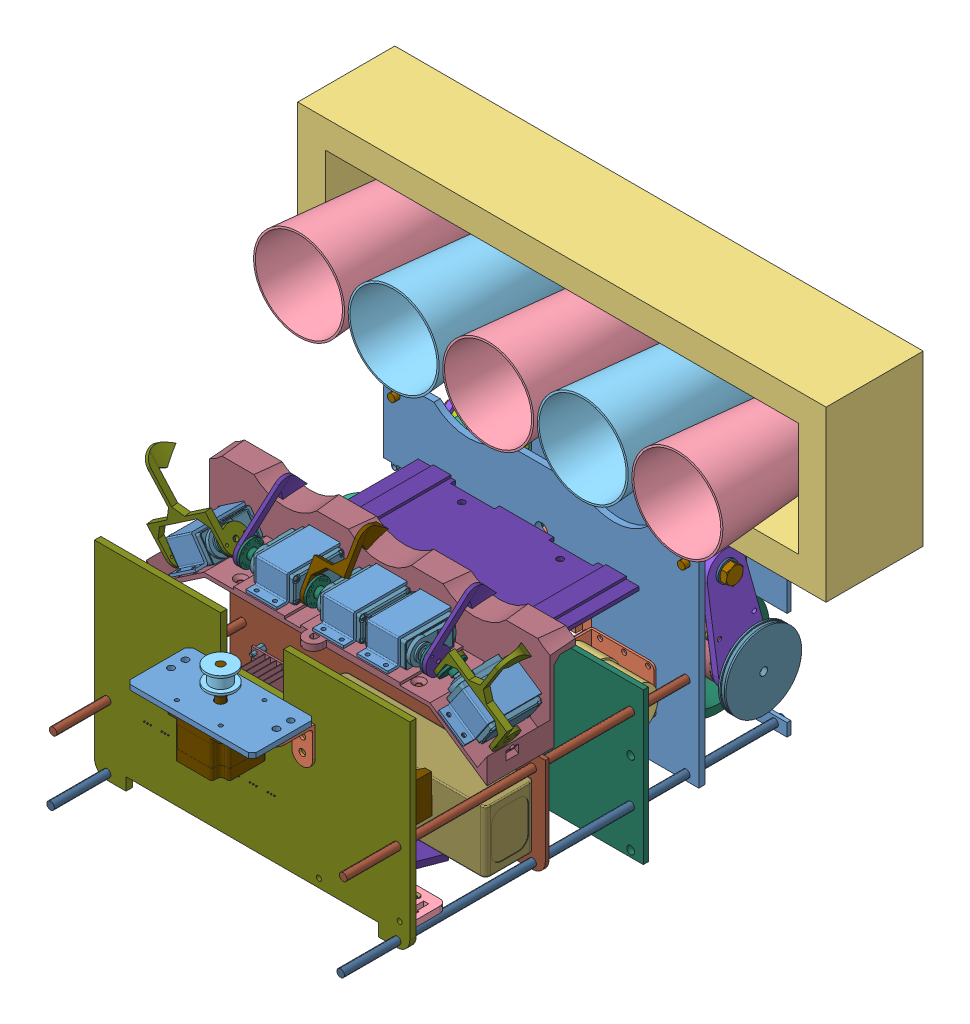
SolidWorks assembly Assemblage ROBOT SGHIR, configuration Default. Lengths in mm. (continued)
Mates (geometry in assembly coordinates): (continued)
- Coaxiale11: concentric: cylinder of assembly; cylinder of assembly; cylinder of baseee-1 through (112.6987 72.7954 187.5605) axis (0 0 1) radius 2; cylinder of support_roulement-4 through (112.6987 72.7954 192.5605) axis (0 0 1) radius 2
- Coaxiale12: concentric: cylinder of assembly; cylinder of assembly; cylinder of baseee-1 through (112.6987 107.7954 187.5605) axis (0 0 1) radius 2; cylinder of support_roulement-4 through (112.6987 107.7954 192.5605) axis (0 0 1) radius 2
- Coaxiale13: concentric: cylinder of assembly; cylinder of assembly; cylinder of support_roulement-3 through (148.0987 90.2954 212.5605) axis (-1 0 0) radius 9.5; cylinder of roulement-1 through (142.0987 90.2954 212.5605) axis (1 0 0) radius 9.5
- Coïncidente7: coincident: plane of assembly; plane of assembly; plane of support_roulement-3 through (148.0987 90.2954 212.5605) normal (-1 0 0); plane of roulement-1 through (148.0987 90.2954 212.5605) normal (1 0 0)
- Coaxiale14: concentric: cylinder of assembly; cylinder of assembly; cylinder of support_roulement-4 through (110.6987 90.2954 212.5605) axis (1 0 0) radius 9.5; cylinder of roulement-2 through (110.6987 90.2954 212.5605) axis (1 0 0) radius 9.5
- Coïncidente8: coincident: plane of assembly; plane of assembly; plane of support_roulement-4 through (110.6987 90.2954 212.5605) normal (1 0 0); plane of roulement-2 through (110.6987 90.2954 212.5605) normal (-1 0 0)
- Coïncidente10: coincident: plane of assembly; plane of assembly; plane of support_roulement-2 through (101.4987 90.2954 212.5605) normal (-1 0 0); plane of roulement-3 through (101.4987 90.2954 212.5605) normal (1 0 0)
- Coaxiale15: concentric: cylinder of assembly; cylinder of assembly; cylinder of support_roulement-2 through (101.4987 90.2954 212.5605) axis (-1 0 0) radius 9.5; cylinder of roulement-3 through (95.4987 90.2954 212.5605) axis (1 0 0) radius 9.5
- Coaxiale16: concentric: cylinder of assembly; cylinder of assembly; cylinder of support_roulement-1 through (62.0987 90.2954 212.5605) axis (1 0 0) radius 7.5; cylinder of roulement-4 through (64.0987 90.2954 212.5605) axis (1 0 0) radius 9.5
- Coïncidente11: coincident: plane of assembly; plane of assembly; plane of support_roulement-1 through (64.0987 90.2954 212.5605) normal (1 0 0); plane of roulement-4 through (64.0987 90.2954 212.5605) normal (-1 0 0)
- Coaxiale17: concentric: cylinder of assembly; cylinder of assembly; cylinder of roulement-4 through (70.0987 90.2954 212.5605) axis (-1 0 0) radius 3; cylinder of axe de tombour-1 through (53.6516 90.2954 212.5605) axis (1 0 0) radius 3
- Coaxiale18: concentric: cylinder of assembly; cylinder of assembly; cylinder of axe de tombour-1 through (53.6516 90.2954 212.5605) axis (1 0 0) radius 3; cylinder of small_roue-1 through (87.1298 90.2954 212.5605) axis (-1 0 0) radius 3.025
- Coaxiale19: concentric: cylinder of assembly; cylinder of assembly; cylinder of roulement-1 through (148.0987 90.2954 212.5605) axis (-1 0 0) radius 3; cylinder of axe de tombour-2 through (115.8668 90.2954 212.5605) axis (1 0 0) radius 3
- Coaxiale20: concentric: cylinder of assembly; cylinder of assembly; cylinder of axe de tombour-2 through (115.8668 90.2954 212.5605) axis (1 0 0) radius 3; cylinder of small_roue-2 through (134.9437 90.2954 212.5605) axis (-1 0 0) radius 11.55
- Coïncidente13: coincident: plane of assembly; plane of assembly; plane of baseee-1 through (-18.9013 250.2954 192.5605) normal (0 0 1); plane of supportencodeur+encodeur+roue-1/Part1-1 through (183.7987 185.7954 192.5605) normal (0 0 -1)
- Coaxiale28: concentric: cylinder of assembly; cylinder of assembly; cylinder of baseee-1 through (191.2987 179.7954 179.5605) axis (0 0 1) radius 2; cylinder of supportencodeur+encodeur+roue-1/Part1-1 through (191.2987 179.7954 187.5605) axis (0 0 1) radius 2
- Coaxiale29: concentric: cylinder of assembly; cylinder of assembly; cylinder of baseee-1 through (191.2987 141.7954 179.5605) axis (0 0 1) radius 2; cylinder of supportencodeur+encodeur+roue-1/Part1-1 through (191.2987 141.7954 187.5605) axis (0 0 1) radius 2
- Coïncidente14: coincident: plane of assembly; plane of assembly; plane of Tombour-1 through (162.0768 101.9937 216.965) normal (-1 0 0); plane of Motor Cople-1 through (162.0768 102.9954 212.5605) normal (1 0 0)
- Coaxiale30: concentric: circle of assembly; circle of assembly; circle of Tombour-1; circle of Motor Cople-1
- Coaxiale31: concentric: cylinder of assembly; cylinder of assembly; cylinder of axe de tombour-2 through (115.8668 90.2954 212.5605) axis (1 0 0) radius 3; cylinder of Motor Cople-1 through (162.0768 90.2954 212.5605) axis (-1 0 0) radius 3
- Distance1: distance = 3 mm: plane of assembly; plane of assembly; plane of axe de tombour-2 through (155.8668 90.2954 212.5605) normal (1 0 0); plane of Motor Cople-1 through (152.8668 90.2954 212.5605) normal (-1 0 0)
- Coïncidente15: coincident: plane of baseee-1 through (-18.9013 250.2954 192.5605) normal (0 0 1); plane of Tombour + levier gauche-2/supportencodeur+encodeur+roue-1/Part1-1 through (28.3987 135.7954 192.5605) normal (0 0 -1)
- Coïncidente16: coincident: cylinder of baseee-1 through (20.8987 179.7954 179.5605) axis (0 0 1) radius 2; circle of Tombour + levier gauche-2/supportencodeur+encodeur+roue-1/Part1-1
- Coïncidente17: coincident: circle of baseee-1; cylinder of Tombour + levier gauche-2/supportencodeur+encodeur+roue-1/Part1-1 through (20.8987 141.7954 187.5605) axis (0 0 1) radius 2
- Coaxiale32: concentric: unknown of ?; unknown of Tombour-2
- Coaxiale35: concentric: circle of assembly; cylinder of assembly; circle of Tombour-2; cylinder of accouplement moteur-1 through (50.3307 90.2954 212.5605) axis (-1 0 0) radius 12.5
- Coïncidente20: coincident: plane of assembly; plane of assembly; plane of Tombour-2 through (50.3307 96.4111 223.4622) normal (1 0 0); plane of accouplement moteur-1 through (50.3307 93.2954 212.5605) normal (-1 0 0)
- Coaxiale36: concentric: cylinder of assembly; circle of assembly; cylinder of axe de tombour-1 through (53.6516 90.2954 212.5605) axis (1 0 0) radius 3; circle of Tombour-2
- Coïncidente21: coincident: plane of assembly; plane of assembly; plane of baseee-1 through (-18.9013 250.2954 189.5605) normal (0 0 -1); plane of scroll 04-1 through (77.2489 172.6222 189.5605) normal (0 0 1)
- Coïncidente22: coincident: plane of assembly; plane of assembly; plane of etage moutourat-1 through (-18.9013 200.2954 262.5605) normal (0 0 1); plane of moteurKacem+support-1/supportMoteur-1 through (65.9987 73.2954 262.5605) normal (0 0 -1)
- Coaxiale38: concentric: cylinder of assembly; cylinder of assembly; cylinder of etage moutourat-1 through (57.5987 76.2954 232.6105) axis (0 0 1) radius 2; cylinder of moteurKacem+support-1/supportMoteur-1 through (57.5987 76.2954 300.5605) axis (0 0 -1) radius 2
- Coaxiale39: concentric: cylinder of assembly; circle of assembly; cylinder of moteurKacem+support-2/supportMoteur-1 through (154.5987 105.7954 300.5605) axis (0 0 -1) radius 2; circle of etage moutourat-1
- Coïncidente23: coincident: plane of assembly; plane of assembly; plane of etage moutourat-1 through (-18.9013 200.2954 262.5605) normal (0 0 1); plane of moteurKacem+support-2/supportMoteur-1 through (146.1987 108.7954 262.5605) normal (0 0 -1)
- Parallèle2: parallel: plane of assembly; plane of assembly; plane of etage moutourat-1 through (66.0987 115.2954 227.5605) normal (1 0 0); plane of moteurKacem+support-1/supportMoteur-1 through (65.9987 73.2954 303.2605) normal (1 0 0)
- Parallèle3: parallel: plane of assembly; plane of assembly; plane of etage moutourat-1 through (146.0987 115.2954 227.5605) normal (-1 0 0); plane of moteurKacem+support-2/supportMoteur-1 through (146.1987 108.7954 303.2605) normal (-1 0 0)
- Coïncidente27: coincident: plane of assembly; plane of assembly; plane of etage moutourat-1 through (-18.9013 200.2954 257.5605) normal (0 0 -1); plane of support servo allu-2 through (-18.9013 142.4885 257.5605) normal (0 0 1)
- Coaxiale41: concentric: cylinder of ? through (11.0987 127.5525 248.5605) axis (0 1 0) radius 3; circle of ServoAttacment2-1
- Coïncidente36: coincident: plane of ? through (11.0987 131.0525 248.5605) normal (0 -1 0); plane of ? through (11.0987 131.0525 248.5605) normal (0 1 0)
- Parallèle14: parallel: plane of etage moutourat-1 through (-18.9013 200.2954 262.5605) normal (0 0 1); plane of ? through (3.0987 136.5525 238.5605) normal (0 0 -1)
- Coaxiale44: concentric: circle of assembly; circle of assembly; circle of ServoAttacment2-1; circle of bras manche a air-1
- Coïncidente46: coincident: plane of assembly; plane of assembly; plane of ServoAttacment2-1 through (31.0987 125.0525 248.5605) normal (0 -1 0); plane of bras manche a air-1 through (28.9422 125.0525 250.6459) normal (0 1 0)
- Coïncidente47: coincident: plane of assembly; plane of assembly; plane of ServoAttacment2-1 through (31.0987 127.0525 248.5605) normal (0.695152 0 0.718863); plane of bras manche a air-1 through (28.9422 121.0525 250.6459) normal (0.695152 0 0.718863)
- Parallèle16: parallel: plane of assembly; plane of assembly; plane of baseee-1 through (-18.9013 250.2954 192.5605) normal (0 0 1); plane of etage moutourat-1 through (-18.9013 200.2954 257.5605) normal (0 0 -1)
- Coïncidente52: coincident: plane of assembly; plane of assembly; plane of baseee-1 through (-18.9013 40.2954 192.5605) normal (0 -1 0); plane of etage moutourat-1 through (-18.9013 40.2954 262.5605) normal (0 -1 0)
- Coïncidente54: coincident: plane of assembly; plane of assembly; plane of baseee-1 through (-18.9013 250.2954 192.5605) normal (-1 0 0); plane of etage moutourat-1 through (-18.9013 200.2954 262.5605) normal (-1 0 0)
- Coaxiale45: concentric: cylinder of assembly; cylinder of assembly; cylinder of moteurKacem+support-2/moteurKacem-1 through (125.8987 89.7954 276.2744) axis (1 0 0) radius 3; cylinder of small_roue-3 through (139.7987 89.7954 276.2744) axis (-1 0 0) radius 3.025
- Coïncidente55: coincident: plane of assembly; plane of assembly; plane of moteurKacem+support-2/moteurKacem-1 through (125.8987 89.7954 276.2744) normal (-1 0 0); plane of small_roue-3 through (125.8987 89.7954 276.2744) normal (-1 0 0)
- Coaxiale46: concentric: cylinder of assembly; cylinder of assembly; cylinder of moteurKacem+support-1/moteurKacem-1 through (86.2987 92.2954 276.2744) axis (-1 0 0) radius 3; cylinder of small_roue-4 through (72.3987 92.2954 276.2744) axis (1 0 0) radius 3.025
- Coïncidente56: coincident: plane of assembly; plane of assembly; plane of moteurKacem+support-1/moteurKacem-1 through (86.2987 92.2954 276.2744) normal (1 0 0); plane of small_roue-4 through (86.2987 92.2954 276.2744) normal (1 0 0)
- Coïncidente57: coincident: plane of assembly; plane of assembly; plane of etage moutourat-1 through (-18.9013 200.2954 262.5605) normal (-1 0 0); plane of support servo allu-2 through (-18.9013 142.4885 238.5605) normal (-1 0 0)
- Coaxiale47: concentric: cylinder of assembly; cylinder of assembly; cylinder of support_roulement-1 through (66.0987 72.7954 232.5605) axis (0 0 -1) radius 2; cylinder of vis fixation tambour-1 through (66.0987 72.7954 257.5605) axis (0 0 1) radius 1.5
- Coïncidente58: coincident: plane of assembly; plane of assembly; plane of baseee-1 through (-18.9013 250.2954 189.5605) normal (0 0 -1); plane of vis fixation tambour-1 through (68.5987 72.7954 189.5605) normal (0 0 1)
- Coaxiale48: concentric: cylinder of assembly; cylinder of assembly; cylinder of support_roulement-1 through (66.0987 107.7954 232.5605) axis (0 0 -1) radius 2; cylinder of vis fixation tambour-2 through (66.0987 107.7954 257.5605) axis (0 0 1) radius 1.5
- Coaxiale49: concentric: cylinder of assembly; cylinder of assembly; cylinder of support_roulement-2 through (99.4987 72.7954 232.5605) axis (0 0 -1) radius 2; cylinder of vis fixation tambour-3 through (99.4987 72.7954 257.5605) axis (0 0 1) radius 1.5
- Coaxiale50: concentric: cylinder of assembly; cylinder of assembly; cylinder of support_roulement-2 through (99.4987 107.7954 232.5605) axis (0 0 -1) radius 2; cylinder of vis fixation tambour-4 through (99.4987 107.7954 257.5605) axis (0 0 1) radius 1.5
- Coïncidente59: coincident: plane of assembly; plane of assembly; plane of baseee-1 through (-18.9013 250.2954 189.5605) normal (0 0 -1); plane of vis fixation tambour-2 through (68.5987 107.7954 189.5605) normal (0 0 1)
- Coïncidente60: coincident: plane of assembly; plane of assembly; plane of baseee-1 through (-18.9013 250.2954 189.5605) normal (0 0 -1); plane of vis fixation tambour-3 through (101.9987 72.7954 189.5605) normal (0 0 1)
- Coïncidente61: coincident: plane of assembly; plane of assembly; plane of baseee-1 through (-18.9013 250.2954 189.5605) normal (0 0 -1); plane of vis fixation tambour-4 through (101.9987 107.7954 189.5605) normal (0 0 1)
- Coïncidente62: coincident: plane of vis fixation tambour-4 through (99.4987 107.7954 257.5605) normal (0 1 0); plane of ? through (79.7917 107.7954 230.4096) normal (0 -1 0)
- Coïncidente63: coincident: plane of vis fixation tambour-4 through (99.4987 107.7954 257.5605) normal (0 1 0); plane of ? through (79.7917 107.7954 230.4096) normal (0 -1 0)
- Coaxiale51: concentric: circle of assembly; line of assembly; line of vis fixation tambour-2; line of ressort-1 through (66.0987 107.7954 252.5605) axis (0 0 -1)
- Distance2: distance = 5 mm: point of assembly; plane of assembly; point of ressort-1; plane of vis fixation tambour-2 through (67.5987 107.7954 257.5605) normal (0 0 1)
- Coaxiale52: concentric: circle of assembly; line of assembly; circle of vis fixation tambour-4; line of ressort-2 through (99.4987 107.7954 253.5605) axis (0 0 -1)
- Distance3: distance = 4 mm: point of assembly; plane of assembly; point of ressort-2; plane of vis fixation tambour-4 through (100.9987 107.7954 257.5605) normal (0 0 1)
- Coïncidente66: coincident: plane of assembly; point of assembly; plane of vis fixation tambour-1 through (67.5987 72.7954 257.5605) normal (0 0 1); point of ressort-4
- Coaxiale53: concentric: circle of assembly; line of assembly; circle of vis fixation tambour-1; line of ressort-4 through (66.0987 72.7954 257.5605) axis (0 0 -1)
- Coaxiale54: concentric: circle of assembly; line of assembly; circle of vis fixation tambour-3; line of ressort-3 through (99.4987 72.7954 253.5605) axis (0 0 -1)
- Distance4: distance = 4 mm: point of assembly; plane of assembly; point of ressort-3; plane of vis fixation tambour-3 through (100.9987 72.7954 257.5605) normal (0 0 1)
- Coaxiale55: concentric: cylinder of assembly; cylinder of assembly; cylinder of support_roulement-4 through (112.6987 72.7954 192.5605) axis (0 0 1) radius 2; cylinder of vis fixation tambour-6 through (112.6987 72.7954 257.5605) axis (0 0 1) radius 1.5
- Coaxiale56: concentric: cylinder of assembly; cylinder of assembly; cylinder of support_roulement-4 through (112.6987 107.7954 192.5605) axis (0 0 1) radius 2; cylinder of vis fixation tambour-5 through (112.6987 107.7954 257.5605) axis (0 0 1) radius 1.5
- Coïncidente69: coincident: plane of assembly; plane of assembly; plane of baseee-1 through (-18.9013 250.2954 189.5605) normal (0 0 -1); plane of vis fixation tambour-5 through (115.1987 107.7954 189.5605) normal (0 0 1)
- Coïncidente70: coincident: plane of assembly; plane of assembly; plane of baseee-1 through (-18.9013 250.2954 189.5605) normal (0 0 -1); plane of vis fixation tambour-6 through (115.1987 72.7954 189.5605) normal (0 0 1)
- Coaxiale57: concentric: cylinder of assembly; cylinder of assembly; cylinder of baseee-1 through (146.0987 107.7954 187.5605) axis (0 0 1) radius 2; cylinder of vis fixation tambour-8 through (146.0987 107.7954 257.5605) axis (0 0 1) radius 1.5
- Coaxiale58: concentric: cylinder of assembly; cylinder of assembly; cylinder of baseee-1 through (146.0987 72.7954 187.5605) axis (0 0 1) radius 2; cylinder of vis fixation tambour-7 through (146.0987 72.7954 257.5605) axis (0 0 1) radius 1.5
- Coïncidente71: coincident: plane of assembly; plane of assembly; plane of baseee-1 through (-18.9013 250.2954 189.5605) normal (0 0 -1); plane of vis fixation tambour-8 through (148.5987 107.7954 189.5605) normal (0 0 1)
- Coïncidente72: coincident: plane of assembly; plane of assembly; plane of baseee-1 through (-18.9013 250.2954 189.5605) normal (0 0 -1); plane of vis fixation tambour-7 through (148.5987 72.7954 189.5605) normal (0 0 1)
- Coaxiale59: concentric: line of assembly; circle of assembly; line of ressort-5 through (112.6987 72.7954 253.5605) axis (0 0 -1); circle of vis fixation tambour-6
- Distance5: distance = 4 mm: point of assembly; plane of assembly; point of ressort-5; plane of vis fixation tambour-6 through (114.1987 72.7954 257.5605) normal (0 0 1)
- Coaxiale60: concentric: circle of assembly; line of assembly; circle of vis fixation tambour-5; line of ressort-6 through (112.6987 107.7954 253.5605) axis (0 0 -1)
- Distance6: distance = 4 mm: point of assembly; plane of assembly; point of ressort-6; plane of vis fixation tambour-5 through (114.1987 107.7954 257.5605) normal (0 0 1)
- Coaxiale61: concentric: circle of assembly; line of assembly; circle of vis fixation tambour-8; line of ressort-7 through (146.0987 107.7954 253.5605) axis (0 0 -1)
- Distance7: distance = 4 mm: point of assembly; plane of assembly; point of ressort-7; plane of vis fixation tambour-8 through (147.5987 107.7954 257.5605) normal (0 0 1)
- Coaxiale62: concentric: circle of assembly; line of assembly; circle of vis fixation tambour-7; line of ressort-8 through (146.0987 72.7954 253.5605) axis (0 0 -1)
- Distance8: distance = 4 mm: plane of assembly; point of assembly; plane of vis fixation tambour-7 through (147.5987 72.7954 257.5605) normal (0 0 1); point of ressort-8
- Coaxiale63: concentric: cylinder of vis fixation tambour-7 through (146.0987 72.7954 257.5605) axis (0 0 1) radius 1.5; cylinder of ? through (146.0987 72.7954 254.2311) axis (0 0 -1) radius 0.75
- Distance12: distance = 150 mm: plane of assembly; plane of assembly; plane of etage moutourat-1 through (-18.9013 200.2954 257.5605) normal (0 0 -1); plane of baseee-1 through (-18.9013 250.2954 192.5605) normal (0 0 1)
- Coaxiale64: concentric: cylinder of assembly; cylinder of assembly; cylinder of vis fixation tambour-2 through (66.0987 107.7954 257.5605) axis (0 0 1) radius 1.5; cylinder of rondelle-1 through (66.0987 107.7954 253.5605) axis (0 0 -1) radius 2
- Distance13: distance = 4 mm: plane of assembly; plane of assembly; plane of vis fixation tambour-2 through (67.5987 107.7954 257.5605) normal (0 0 1); plane of rondelle-1 through (66.0987 107.7954 253.5605) normal (0 0 1)
- Coaxiale65: concentric: circle of vis fixation tambour-2; line of ? through (66.0987 107.7954 253.5605) axis (0 0 -1)
- Distance14: distance = 3 mm: plane of assembly; plane of assembly; plane of vis fixation tambour-2 through (67.5987 107.7954 257.5605) normal (0 0 1); plane of salim écrou-1 through (65.7102 107.8336 252.7883) normal (0 0 1)
- Coïncidente87: coincident: plane of ? through (-18.9013 40.2954 347.5605) normal (0 -1 0); plane of ? through (-8.9013 40.2954 410.5605) normal (0 -1 0)
- Coïncidente88: coincident: plane of ? through (-18.9013 200.2954 347.5605) normal (-1 0 0); plane of ? through (-18.9013 120.2954 410.5605) normal (-1 0 0)
- Distance16: distance = 60 mm: plane of assembly; plane of assembly; plane of 3 etage-1 through (-8.9013 50.2954 381.2939) normal (0 0 -1); plane of etage moutourat-1 through (-18.9013 200.2954 262.5605) normal (0 0 1)
- Coïncidente90: coincident: plane of ? through (-8.9013 50.2954 410.5605) normal (0 0 1); plane of ? through (153.6734 75.7626 410.5605) normal (0 0 -1)
- Distance20: distance = 5 mm: plane of assembly; plane of assembly; plane of 3 etage-1 through (-8.9013 50.2954 384.2939) normal (0 0 1); plane of L298N Motor Driver-1 through (26.3982 67.0454 389.2939) normal (0 0 -1)
- Distance17: distance = 13.4672 mm: plane of assembly; plane of assembly; plane of 3 etage-1 through (-8.9013 40.2954 384.2939) normal (0 -1 0); plane of Lipot 5000 mAh-1 through (222.6734 53.7626 423.2939) normal (0 -1 0)
- Distance18: distance = 5.8205 mm: plane of assembly; plane of assembly; plane of 3 etage-1 through (-8.9013 40.2954 384.2939) normal (0 -1 0); plane of L298N Motor Driver-1 through (48.1482 45.2954 390.7939) normal (0 -1 0)
- Distance19: distance = 25.8542 mm: plane of assembly; plane of assembly; plane of 3 etage-1 through (-18.9013 120.2954 384.2939) normal (-1 0 0); plane of L298N Motor Driver-1 through (4.6482 88.7954 390.7939) normal (-1 0 0)
- Coaxiale66: concentric: cylinder of ? through (9.953 86.616 417.0605) axis (0 0 -1) radius 1.5; cylinder of ? through (9.953 86.616 415.5605) axis (0 0 1) radius 1.5
- Parallèle19: parallel: cylinder of ? through (9.953 49.116 417.0605) axis (0 0 -1) radius 1.5; cylinder of ? through (47.453 86.616 415.5605) axis (0 0 1) radius 1.5
- Coaxiale67: concentric: cylinder of ? through (47.453 49.116 417.0605) axis (0 0 -1) radius 1.5; cylinder of ? through (47.453 49.116 415.5605) axis (0 0 1) radius 1.5
- Coïncidente99: coincident: plane of ? through (28.703 67.866 415.5605) normal (0 0 -1); plane of ? through (47.3375 49.1826 415.5605) normal (0 0 1)
- Coïncidente100: coincident: plane of ? through (28.703 67.866 415.5605) normal (0 0 -1); plane of ? through (9.953 86.4826 415.5605) normal (0 0 1)
- Coaxiale68: concentric: cylinder of ? through (47.453 86.616 417.0605) axis (0 0 -1) radius 1.5; cylinder of ? through (47.453 86.616 415.5605) axis (0 0 1) radius 1.5
- Parallèle20: parallel: cylinder of ? through (9.953 49.116 417.0605) axis (0 0 -1) radius 1.5; cylinder of ? through (47.453 86.616 415.5605) axis (0 0 1) radius 1.5
- Coaxiale70: concentric: cylinder of ? through (9.953 49.116 417.0605) axis (0 0 -1) radius 1.5; cylinder of ? through (9.953 49.116 415.5605) axis (0 0 1) radius 1.5
- Coïncidente101: coincident: plane of ? through (28.703 67.866 415.5605) normal (0 0 -1); plane of ? through (10.0685 49.1826 415.5605) normal (0 0 1)
- Coïncidente102: coincident: plane of ? through (28.703 67.866 415.5605) normal (0 0 -1); plane of ? through (47.453 86.4826 415.5605) normal (0 0 1)
- Coïncidente103: coincident: plane of assembly; plane of assembly; plane of etage moutourat-1 through (-18.9013 40.2954 262.5605) normal (0 -1 0); plane of 3 etage-1 through (-8.9013 40.2954 384.2939) normal (0 -1 0)
- Coïncidente104: coincident: plane of assembly; plane of assembly; plane of etage moutourat-1 through (-18.9013 200.2954 262.5605) normal (-1 0 0); plane of 3 etage-1 through (-18.9013 120.2954 384.2939) normal (-1 0 0)
- Coaxiale71: concentric: circle of assembly; cylinder of assembly; circle of L298N Motor Driver-1; cylinder of entretoise-3 through (7.6482 48.2954 389.2939) axis (0 0 1) radius 1.5
- Coïncidente105: coincident: plane of assembly; plane of assembly; plane of L298N Motor Driver-1 through (26.3982 67.0454 389.2939) normal (0 0 -1); plane of entretoise-3 through (7.7636 48.3621 389.2939) normal (0 0 1)
- Coïncidente106: coincident: plane of assembly; plane of assembly; plane of L298N Motor Driver-1 through (26.3982 67.0454 389.2939) normal (0 0 -1); plane of entretoise-1 through (7.5152 85.7854 389.2939) normal (0 0 1)
- Coaxiale72: concentric: cylinder of assembly; cylinder of assembly; cylinder of L298N Motor Driver-1 through (7.6482 85.7954 390.7939) axis (0 0 -1) radius 1.5; cylinder of entretoise-1 through (7.6482 85.7954 389.2939) axis (0 0 1) radius 1.5
- Coaxiale73: concentric: cylinder of assembly; cylinder of assembly; cylinder of L298N Motor Driver-1 through (45.1482 48.2954 390.7939) axis (0 0 -1) radius 1.5; cylinder of entretoise-2 through (45.1482 48.2954 389.2939) axis (0 0 1) radius 1.5
- Coïncidente107: coincident: plane of assembly; plane of assembly; plane of L298N Motor Driver-1 through (26.3982 67.0454 389.2939) normal (0 0 -1); plane of entretoise-2 through (45.0327 48.3621 389.2939) normal (0 0 1)
- Coaxiale74: concentric: cylinder of assembly; cylinder of assembly; cylinder of L298N Motor Driver-1 through (45.1482 85.7954 390.7939) axis (0 0 -1) radius 1.5; cylinder of entretoise-4 through (45.1482 85.7954 389.2939) axis (0 0 1) radius 1.5
- Coïncidente108: coincident: plane of assembly; plane of assembly; plane of L298N Motor Driver-1 through (26.3982 67.0454 389.2939) normal (0 0 -1); plane of entretoise-4 through (45.0152 85.7854 389.2939) normal (0 0 1)
- Coïncidente109: coincident: plane of assembly; plane of assembly; plane of 3 etage-1 through (-8.9013 50.2954 384.2939) normal (0 0 1); plane of entretoise-1 through (7.5152 85.7854 384.2939) normal (0 0 -1)
- Coïncidente110: coincident: plane of assembly; plane of assembly; plane of 3 etage-1 through (-8.9013 50.2954 384.2939) normal (0 0 1); plane of Lipot 5000 mAh-1 through (153.6734 75.7626 384.2939) normal (0 0 -1)
- Distance21: distance = 5 mm: plane of assembly; plane of assembly; plane of 3 etage-1 through (-8.9013 40.2954 384.2939) normal (0 -1 0); plane of L298N Motor Driver-1 through (48.1482 45.2954 390.7939) normal (0 -1 0)
- Coaxiale75: concentric: circle of assembly; cylinder of assembly; circle of L298N Motor Driver-1; cylinder of entretoise-1 through (7.6482 85.7954 389.2939) axis (0 0 1) radius 1.5
- Coïncidente114: coincident: plane of assembly; plane of assembly; plane of etage moutourat-1 through (-18.9013 200.2954 262.5605) normal (-1 0 0); plane of étage servo-1 through (-18.9013 129.7933 306.5605) normal (-1 0 0)
- Parallèle26: parallel: cylinder of assembly; cylinder of assembly; cylinder of 3 etage-1 through (45.1482 48.2954 374.2939) axis (0 0 1) radius 1.4252; cylinder of entretoise-2 through (45.1482 48.2954 389.2939) axis (0 0 1) radius 1.5
- Coïncidente136: coincident: plane of assembly; plane of assembly; plane of 3 etage-1 through (-8.9013 40.2954 384.2939) normal (0 -1 0); plane of etage electro-1 through (221.0987 40.2954 491.706) normal (0 -1 0)
- Parallèle28: parallel: plane of assembly; plane of assembly; plane of 3 etage-1 through (-8.9013 50.2954 384.2939) normal (0 0 1); plane of etage electro-1 through (221.0987 50.2954 486.706) normal (0 0 -1)
- Coïncidente138: coincident: plane of assembly; plane of assembly; plane of 3 etage-1 through (231.0987 120.2954 384.2939) normal (1 0 0); plane of etage electro-1 through (231.0987 50.2954 491.706) normal (1 0 0)
- Coïncidente139: coincident: plane of assembly; plane of assembly; plane of etage electro-1 through (221.0987 50.2954 486.706) normal (0 0 -1); plane of support servo allu-3 through (151.0987 61.9278 486.706) normal (0 0 1)
- Parallèle30: parallel: plane of ? through (221.0987 50.2954 463.3946) normal (0 0 -1); plane of ? through (209.9589 56.7954 497.1289) normal (0 0 1)
- Coaxiale85: concentric: cylinder of assembly; cylinder of assembly; cylinder of 3alam-1 through (201.0987 40.2954 477.706) axis (0 1 0) radius 2; cylinder of ServoAttacment2-3 through (201.0987 51.2954 477.706) axis (0 -1 0) radius 4
- Coïncidente142: coincident: plane of assembly; plane of assembly; plane of 3alam-1 through (66.7107 45.2954 431.5663) normal (0 1 0); plane of ServoAttacment2-3 through (201.0987 45.2954 477.706) normal (0 -1 0)
- Parallèle32: parallel: plane of assembly; plane of assembly; plane of 3alam-1 through (66.7107 40.2954 431.5663) normal (0.357807 0 -0.933796); plane of ServoAttacment2-3 through (201.0987 47.2954 477.706) normal (-0.357807 0 0.933796)
- Coaxiale86: concentric: cylinder of ? through (201.9589 47.7954 487.1289) axis (0 1 0) radius 3; cylinder of ? through (201.9589 51.2954 487.1289) axis (0 -1 0) radius 4
- Coïncidente145: coincident: plane of ? through (201.9589 51.2954 487.1289) normal (0 -1 0); plane of ? through (201.9589 51.2954 487.1289) normal (0 1 0)
- Coïncidente146: coincident: plane of assembly; plane of assembly; plane of etage electro-1 through (221.0987 40.2954 491.706) normal (0 -1 0); plane of 3alam-1 through (66.7107 40.2954 431.5663) normal (0 -1 0)
- Coïncidente147: coincident: plane of assembly; plane of assembly; plane of etage electro-1 through (231.0987 50.2954 491.706) normal (1 0 0); plane of support servo allu-3 through (231.0987 61.9278 486.706) normal (1 0 0)
- Distance22: distance = 15 mm: plane of assembly; plane of assembly; plane of TB6560 Stepper driver-1 through (173.9926 122.1069 471.706) normal (0 0 1); plane of etage electro-1 through (221.0987 50.2954 486.706) normal (0 0 -1)
- Distance23: distance = 2.46 mm: plane of assembly; plane of assembly; plane of Carte 8 servos.STEP-1/Layer_1.STEP-1 through (11.2764 117.1304 484.246) normal (0 0 1); plane of etage electro-1 through (221.0987 50.2954 486.706) normal (0 0 -1)
- Parallèle34: parallel: plane of assembly; plane of assembly; plane of etage electro-1 through (231.0987 50.2954 491.706) normal (1 0 0); plane of Carte 8 servos.STEP-1/Layer_1.STEP-1 through (146.2764 117.1304 484.246) normal (1 0 0)
- Largeur7: width: plane of etage moutourat-1 through (231.0987 200.2954 262.5605) normal (1 0 0); plane of etage moutourat-1 through (-18.9013 200.2954 262.5605) normal (-1 0 0); plane of base vertical-1 through (18.5987 162.1523 272.5605) normal (-1 0 0); plane of base vertical-1 through (193.5987 162.1523 392.5605) normal (1 0 0)
- Distance24: distance = 10 mm: plane of etage moutourat-1 through (-18.9013 200.2954 262.5605) normal (0 0 1); plane of base vertical-1 through (48.0987 162.1523 272.5605) normal (0 0 -1)
- Distance25: distance = 40 mm: plane of assembly; plane of assembly; plane of etage moutourat-1 through (-18.9013 200.2954 262.5605) normal (0 0 1); plane of étage servo-1 through (-18.9013 129.7933 302.5605) normal (0 0 -1)
- Parallèle39: parallel: plane of assembly; plane of assembly; plane of etage electro-1 through (221.0987 50.2954 491.706) normal (0 0 1); plane of NEMA34-JK86HS68-5904-1 through (93.0987 152.7954 495.356) normal (0 0 -1)
- Coïncidente158: coincident: plane of assembly; plane of assembly; plane of NEMA34-JK86HS68-5904-1 through (125.4987 161.2954 536.106) normal (0 1 0); plane of support pasàpas-1 through (66.0987 161.2954 541.706) normal (0 -1 0)
- Largeur8: width: plane of assembly; plane of assembly; plane of assembly; plane of assembly; plane of NEMA34-JK86HS68-5904-1 through (84.7487 152.7954 529.706) normal (-1 0 0); plane of NEMA34-JK86HS68-5904-1 through (127.4487 152.7954 503.706) normal (1 0 0); plane of support pasàpas-1 through (156.0987 161.2954 541.706) normal (1 0 0); plane of support pasàpas-1 through (56.0987 161.2954 541.706) normal (-1 0 0)
- Largeur9: width: plane of assembly; plane of assembly; plane of assembly; plane of assembly; plane of NEMA34-JK86HS68-5904-1 through (119.0987 152.7954 538.056) normal (0 0 1); plane of NEMA34-JK86HS68-5904-1 through (93.0987 152.7954 495.356) normal (0 0 -1); plane of support pasàpas-1 through (56.0987 161.2954 491.706) normal (0 0 -1); plane of support pasàpas-1 through (56.0987 161.2954 541.706) normal (0 0 1)
- Coïncidente160: coincident: plane of assembly; plane of assembly; plane of etage electro-1 through (221.0987 50.2954 491.706) normal (0 0 1); plane of grand_l-1 through (139.5987 160.7954 491.706) normal (0 0 -1)
- Coïncidente161: coincident: plane of assembly; plane of assembly; plane of etage electro-1 through (221.0987 50.2954 491.706) normal (0 0 1); plane of grand_l-2 through (56.0987 160.7954 491.706) normal (0 0 -1)
- Largeur10: width: plane of assembly; plane of assembly; plane of assembly; plane of assembly; plane of NEMA34-JK86HS68-5904-1 through (84.7487 152.7954 529.706) normal (-1 0 0); plane of NEMA34-JK86HS68-5904-1 through (127.4487 152.7954 503.706) normal (1 0 0); plane of etage electro-1 through (231.0987 50.2954 491.706) normal (1 0 0); plane of etage electro-1 through (-18.9013 50.2954 491.706) normal (-1 0 0)
- Coïncidente162: coincident: plane of assembly; plane of assembly; plane of etage electro-1 through (131.0987 165.2954 491.706) normal (0 1 0); plane of support pasàpas-1 through (66.0987 165.2954 541.706) normal (0 1 0)
- Parallèle40: parallel: plane of assembly; plane of assembly; plane of etage electro-1 through (131.0987 165.2954 491.706) normal (0 1 0); plane of grand_l-1 through (139.5987 161.2954 492.206) normal (0 1 0)
- Parallèle41: parallel: plane of assembly; plane of assembly; plane of etage electro-1 through (131.0987 165.2954 491.706) normal (0 1 0); plane of grand_l-2 through (56.0987 161.2954 492.206) normal (0 1 0)
- Coïncidente165: coincident: plane of assembly; plane of assembly; plane of support pasàpas-1 through (66.0987 161.2954 541.706) normal (0 -1 0); plane of grand_l-2 through (56.0987 161.2954 492.206) normal (0 1 0)
- Coïncidente166: coincident: plane of assembly; plane of assembly; plane of support pasàpas-1 through (66.0987 161.2954 541.706) normal (0 -1 0); plane of grand_l-1 through (139.5987 161.2954 492.206) normal (0 1 0)
- Coïncidente167: coincident: plane of assembly; plane of assembly; plane of etage electro-1 through (221.0987 50.2954 491.706) normal (0 0 1); plane of support pasàpas-1 through (56.0987 161.2954 491.706) normal (0 0 -1)
- Coïncidente168: coincident: plane of assembly; plane of assembly; plane of support pasàpas-1 through (56.0987 161.2954 541.706) normal (-1 0 0); plane of grand_l-2 through (56.0987 156.2954 496.706) normal (-1 0 0)
- Coïncidente169: coincident: plane of assembly; plane of assembly; plane of support pasàpas-1 through (156.0987 161.2954 541.706) normal (1 0 0); plane of grand_l-1 through (156.0987 156.2954 496.706) normal (1 0 0)
- Coaxiale87: concentric: cylinder of assembly; cylinder of assembly; cylinder of NEMA34-JK86HS68-5904-1 through (106.0836 141.481 516.7322) axis (0 1 0) radius 3.5; cylinder of small_roue-5 through (106.0836 176.331 516.7322) axis (0 1 0) radius 3.025
- Coïncidente170: coincident: plane of NEMA34-JK86HS68-5904-1 through (106.0836 190.231 516.7322) normal (0 1 0); plane of small_roue-5 through (106.0836 190.231 516.7322) normal (0 1 0)
- Coïncidente176: coincident: plane of ? through (-18.9013 40.2954 306.5605) normal (0 -1 0); plane of ? through (167.0987 40.2954 336.5605) normal (0 -1 0)
- Coaxiale90: concentric: cylinder of ? through (153.5987 144.2954 321.5605) axis (0 -1 0) radius 3.5; cylinder of ? through (153.5987 110.2954 321.5605) axis (0 1 0) radius 3.5
- Coïncidente180: coincident: plane of ? through (-18.9013 160.2954 306.5605) normal (0 0 1); plane of ? through (139.0987 118.2954 306.5605) normal (0 0 -1)
- Coïncidente196: coincident: plane of assembly; plane of assembly; plane of eceuil-1 through (-44.4013 268.9793 188.0985) normal (0 0 1); plane of green cup-2 through (-18.9013 268.9793 188.0985) normal (0 0 -1)
- Coaxiale94: concentric: cylinder of eceuil-1 through (-44.4013 268.9793 188.0985) axis (0 0 1) radius 28; circle of green cup-2
- Coïncidente197: coincident: plane of eceuil-1 through (30.5987 268.9793 188.0985) normal (0 0 1); plane of red cup-1 through (56.0987 268.9793 188.0985) normal (0 0 -1)
- Coaxiale95: concentric: cylinder of eceuil-1 through (30.5987 268.9793 188.0985) axis (0 0 1) radius 28; circle of red cup-1
- Coïncidente198: coincident: plane of eceuil-1 through (105.5987 268.9793 188.0985) normal (0 0 1); plane of green cup-1 through (131.0987 268.9793 188.0985) normal (0 0 -1)
- Coaxiale96: concentric: circle of eceuil-1; circle of green cup-1
- Coïncidente199: coincident: plane of eceuil-1 through (180.5987 268.9793 188.0985) normal (0 0 1); plane of red cup-2 through (206.0987 268.9793 188.0985) normal (0 0 -1)
- Coaxiale97: concentric: circle of eceuil-1; circle of red cup-2
- Coïncidente200: coincident: plane of eceuil-1 through (255.5987 268.9793 188.0985) normal (0 0 1); plane of green cup-4 through (281.0987 268.9793 188.0985) normal (0 0 -1)
- Coaxiale98: concentric: cylinder of eceuil-1 through (255.5987 268.9793 188.0985) axis (0 0 1) radius 28; circle of green cup-4
- Distance32: distance = 70 mm: plane of assembly through (0 0 176.0985) normal (0 0 -1); plane of eceuil-1 through (-103.4013 335.9793 246.0985) normal (0 0 1)
- Coïncidente204: coincident: plane of étage servo-1 through (-18.9013 129.7933 306.5605) normal (0 0 1); plane of verin complet-2/body-1 through (118.0987 83.7933 306.5605) normal (0 0 -1)
- Largeur16: width: plane of verin complet-2/body-1 through (118.0987 54.9978 321.5605) normal (1 0 0); plane of verin complet-2/body-1 through (94.0987 54.9978 321.5605) normal (-1 0 0); plane of étage servo-1 through (-18.9013 129.7933 306.5605) normal (-1 0 0); plane of étage servo-1 through (231.0987 129.7933 306.5605) normal (1 0 0)
- Coïncidente205: coincident: plane of étage servo-1 through (-18.9013 9.7933 306.5605) normal (0 -1 0); plane of verin complet-2/body-1 through (118.0987 9.7933 336.5605) normal (0 -1 0)
- Coïncidente206: coincident: plane of ? through (101.8627 171.2954 322.791) normal (-0.912003 0 0.410184); unknown of ?
- Coaxiale99: concentric: cylinder of ? through (95.4139 176.6545 325.6915) axis (0.912003 0 -0.410184) radius 2.5; cylinder of ? through (108.2468 176.6545 319.9197) axis (-0.912003 0 0.410184) radius 2.5
- Coïncidente207: coincident: plane of base vertical-1 through (18.5987 162.1523 392.5605) normal (0 -1 0); plane of support de fixation-1 through (110.5987 162.1523 327.5605) normal (0 1 0)
- Coaxiale100: concentric: cylinder of verin complet-2/body-1 through (104.5987 112.7933 321.5605) axis (0 -1 0) radius 10.5; cylinder of tige-2 through (104.5987 85.7933 321.5605) axis (0 1 0) radius 3.5
- Coïncidente209: coincident: plane of support de fixation-1 through (98.5987 147.1523 318.5605) normal (0 0 1); plane of tige-2 through (104.5987 146.7933 318.5605) normal (0 0 -1)
- Coaxiale101: concentric: cylinder of support de fixation-1 through (104.5987 152.1523 315.5605) axis (0 0 1) radius 2.5; cylinder of tige-2 through (104.5987 152.1523 311.4894) axis (0 0 1) radius 2.5
- Parallèle45: parallel: plane of base vertical-1 through (18.5987 162.1523 392.5605) normal (0 0 1); plane of support de fixation-1 through (119.5987 162.1523 336.5605) normal (0 0 1)
- Largeur17: width: plane of eceuil-1 through (-103.4013 335.9793 191.0985) normal (-1 0 0); plane of eceuil-1 through (315.5987 335.9793 191.0985) normal (1 0 0); plane of etage moutourat-1 through (231.0987 200.2954 262.5605) normal (1 0 0); plane of etage moutourat-1 through (-18.9013 200.2954 262.5605) normal (-1 0 0)
- Coaxiale102: concentric: cylinder of assembly; cylinder of assembly; cylinder of baseee-1 through (-8.9013 190.2954 182.5605) axis (0 0 1) radius 3.1; cylinder of tige pour palier-1 through (-8.9013 190.2954 266.5605) axis (0 0 -1) radius 3
- Distance33: distance = 3 mm: plane of tige pour palier-1 through (-8.9013 190.2954 186.5605) normal (0 0 -1); plane of baseee-1 through (-18.9013 250.2954 189.5605) normal (0 0 -1)
- Coaxiale103: concentric: cylinder of assembly; cylinder of assembly; cylinder of baseee-1 through (221.0987 190.2954 182.5605) axis (0 0 1) radius 3.1; cylinder of tige pour palier-2 through (221.0987 190.2954 266.5605) axis (0 0 -1) radius 3
- Distance34: distance = 3 mm: plane of tige pour palier-2 through (221.0987 190.2954 186.5605) normal (0 0 -1); plane of baseee-1 through (-18.9013 250.2954 189.5605) normal (0 0 -1)
- Coaxiale104: concentric: cylinder of assembly; cylinder of assembly; cylinder of baseee-1 through (221.0987 45.2954 182.5605) axis (0 0 1) radius 3.1; cylinder of grand tige 350mm-1 through (221.0987 45.2954 536.5605) axis (0 0 -1) radius 3
- Distance35: distance = 3 mm: plane of grand tige 350mm-1 through (221.0987 45.2954 186.5605) normal (0 0 -1); plane of baseee-1 through (-18.9013 250.2954 189.5605) normal (0 0 -1)
- Coaxiale105: concentric: cylinder of assembly; cylinder of assembly; cylinder of baseee-1 through (-8.9013 45.2954 182.5605) axis (0 0 1) radius 3.1; cylinder of grand tige 350mm-2 through (-8.9013 45.2954 536.5605) axis (0 0 -1) radius 3
- Distance36: distance = 3 mm: plane of baseee-1 through (-18.9013 250.2954 189.5605) normal (0 0 -1); plane of grand tige 350mm-2 through (-8.9013 45.2954 186.5605) normal (0 0 -1)
- Coaxiale106: concentric: cylinder of assembly; cylinder of assembly; cylinder of etage moutourat-1 through (221.0987 110.2954 267.5605) axis (0 0 -1) radius 3.1; cylinder of tige 280mm-1 through (221.0987 110.2954 534.5605) axis (0 0 -1) radius 3
- Distance37: distance = 3 mm: plane of tige 280mm-1 through (221.0987 110.2954 254.5605) normal (0 0 -1); plane of etage moutourat-1 through (-18.9013 200.2954 257.5605) normal (0 0 -1)
- Coaxiale107: concentric: cylinder of assembly; cylinder of assembly; cylinder of etage moutourat-1 through (-8.9013 95.2954 267.5605) axis (0 0 -1) radius 3.1; cylinder of tige 280mm-2 through (-8.9013 95.2954 534.5605) axis (0 0 -1) radius 3
- Distance38: distance = 3 mm: plane of tige 280mm-2 through (-8.9013 95.2954 254.5605) normal (0 0 -1); plane of etage moutourat-1 through (-18.9013 200.2954 257.5605) normal (0 0 -1)
- Coaxiale108: concentric: cylinder of assembly; cylinder of assembly; cylinder of ServoAttacment2-3 through (201.0987 51.2954 477.706) axis (0 -1 0) radius 4; cylinder of Servo noir-1 through (201.0987 47.7954 477.706) axis (0 1 0) radius 3
- Coïncidente216: coincident: plane of ServoAttacment2-3 through (201.0987 51.2954 477.706) normal (0 1 0); plane of Servo noir-1 through (201.0987 51.2954 477.706) normal (0 -1 0)
- Parallèle46: parallel: plane of etage electro-1 through (221.0987 50.2954 491.706) normal (0 0 1); plane of Servo noir-1 through (209.0987 56.7954 467.706) normal (0 0 -1)
- Coaxiale110: concentric: cylinder of support servo allu-3 through (214.9987 61.9278 482.806) axis (0 -1 0) radius 2.15; cylinder of Servo noir-1 through (214.9987 60.2954 482.806) axis (0 1 0) radius 2.15
- Coaxiale111: concentric: circle of assembly; cylinder of assembly; circle of ServoAttacment2-1; cylinder of Servo noir-2 through (31.0987 129.9885 248.5605) axis (0 1 0) radius 3
- Parallèle47: parallel: plane of etage moutourat-1 through (-18.9013 200.2954 257.5605) normal (0 0 -1); plane of Servo noir-2 through (39.0987 138.9885 258.5605) normal (0 0 1)
- Coaxiale112: concentric: cylinder of support servo allu-2 through (-2.8013 142.4885 243.4605) axis (0 -1 0) radius 2.15; cylinder of Servo noir-2 through (-2.8013 142.4885 243.4605) axis (0 1 0) radius 2.15
- Coïncidente219: coincident: plane of support servo allu-2 through (-13.9013 142.4885 238.5605) normal (0 1 0); plane of Servo noir-2 through (45.7872 142.4885 240.8721) normal (0 -1 0)
- Distance39: distance = 22 mm: plane of tige-2 through (104.5987 135.7933 321.5605) normal (0 -1 0); plane of verin complet-2/body-1 through (104.5987 113.7933 321.5605) normal (0 1 0)
- Coincident1: coincident: plane of base vertical-1 through (18.5987 167.1523 392.5605) normal (0 1 0); plane of new system-1/main-1 through (-28.9013 167.1523 387.4162) normal (0 -1 0)
- Parallel1: parallel: plane of base vertical-1 through (18.5987 162.1523 392.5605) normal (0 0 1); plane of new system-1/main-1 through (-28.9013 167.1523 440.4162) normal (0 0 1)
- Distance40: distance = 87.5 mm: plane of new system-1/main-1 through (106.0987 167.1523 387.4162) normal (-1 0 0); plane of base vertical-1 through (193.5987 162.1523 392.5605) normal (1 0 0)
